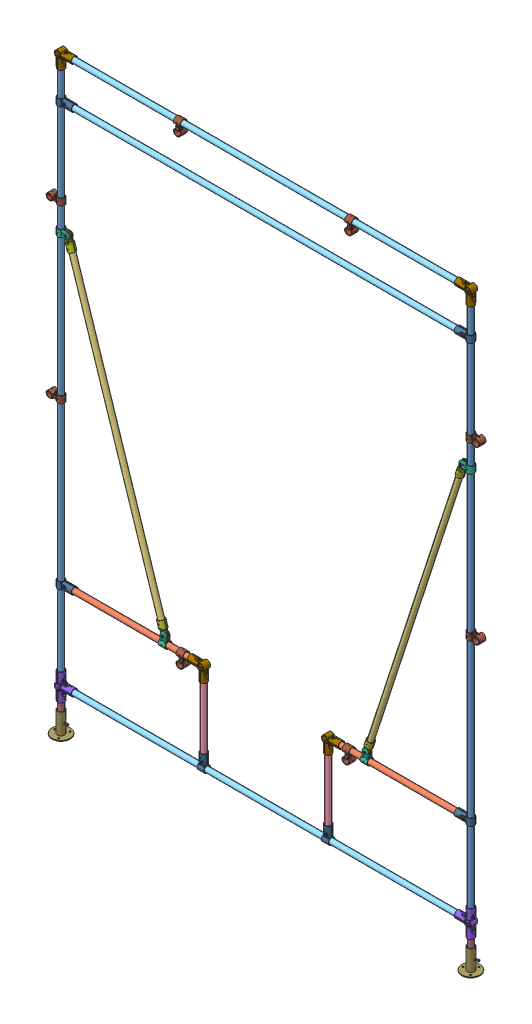
SolidWorks assembly Steel Tube Panel2, configuration Default. Lengths in mm.
Overall size (2121.41 2906.78 107.19).
47 component instances, 13 part files, 77 mates.
Components (placement in the parent):
- Height-1: Height [Default] at (0 2644.14 0) x (0 -1 0) z (0.644967 0 0.76421) size (2606.04 25.4 25.4)
- Horizonal Corner-1: Horizonal Corner [Default] at (1346.2 431.8 0) x (1 0 0) z (0 -0.094646 -0.995511) size (622.3 25.4 25.4)
- Lower Mounting Bar-1: Lower Mounting Bar [Default] at (1508.7506 501.6503 0) x (0.309017 0.951057 0) z (0.758734 -0.246528 0.602949) size (1460.5 25.4 25.4)
- Vertical Corner-1: Vertical Corner [Default] at (1308.1 38.1 0) x (0 1 0) z (-0.861516 0 -0.50773) size (355.6 25.4 25.4)
- Width-1: Width [Default] at (1968.5 0 0) x (-1 0 0) z (0 0.829168 0.559) size (1930.4 25.4 25.4)
- Adjustable_18deg-1: Adjustable_18deg [Default] at (1936.0393 1953.3743 -8.9201) x (-1 0 0) z (0 0 1) size (87.05 82.3 33.53)
  - Adjustable Connector Part 1-1: Adjustable Connector Part 1 [2534T33] at (-70.5607 28.1617 8.9201) size (68.33 33.53 33.53)
  - Adjustable Connector Part 2-1: Adjustable Connector Part 2 [2534T33] at (-46.1648 -5.4163 8.9201) x (0.309017 0.951057 0) z (0 0 1) size (75.66 33.46 33.53)
- Adjustable_72deg-1: Adjustable_72deg [Default] at (1469.3648 502.3607 8.9201) x (0 1 0) z (0 0 -1) size (115.94 55.2 33.53)
  - Adjustable Connector Part 1-1: Adjustable Connector Part 1 [2534T33] at (-70.5607 28.1617 8.9201) size (68.33 33.53 33.53)
  - Adjustable Connector Part 2-1: Adjustable Connector Part 2 [2534T33] at (-68.8327 17.2515 8.9201) x (0.951057 0.309017 0) z (0 0 1) size (75.66 33.46 33.53)
- 5way connector-1: 5way connector [2534T26] x (0 -1 0) z (0 0 -1) size (130.05 82.36 33.46)
- 5way connector-2: 5way connector [2534T26] at (2006.6 0 0) x (0 1 0) z (0 0 -1) size (130.05 82.36 33.46)
- Height-2: Height [Default] at (2006.6 2644.14 0) x (0 -1 0) z (0 0 1) size (2606.04 25.4 25.4)
- 3way connector-2: 3way connector [2534T24] at (2006.6 2682.24 0) x (-1 0 0) z (0 0 -1) size (81.85 81.28 33.46)
- 3way connector-3: 3way connector [2534T24] at (0 2682.24 0) size (81.85 81.28 33.46)
- Width-2: Width [Default] at (1968.5 2682.24 0) x (-1 0 0) z (0 0.006098 -0.999981) size (1930.4 25.4 25.4)
- Tee connector-1: Tee connector [2534T21] at (1308.1 0 0) x (1 0 0) z (0 0 -1) size (33.53 82.55 34.1)
- Tee connector-2: Tee connector [2534T21] at (2006.6 431.8 0) x (0 1 0) z (0 0 -1) size (33.53 82.55 34.1)
- 3way connector-4: 3way connector [2534T24] at (1308.1 431.8 0) size (81.85 81.28 33.46)
- Crossover-1: Crossover [2534T28] at (2006.6 1219.2 0) x (1 0 -0.000006) z (0 -1 0) size (74.17 39.33 39.33)
- Crossover-2: Crossover [2534T28] at (2006.6 2057.4 0) x (1 0 -0.000006) z (0 -1 0) size (74.17 39.33 39.33)
- Crossover-3: Crossover [2534T28] at (1422.4 2682.24 0) x (0 -1 -0.000006) z (-1 0 0) size (74.17 39.33 39.33)
- Tee connector-9: Tee connector [2534T21] at (0 2479.04 0) x (0 1 0) z (0 0 1) size (33.53 82.55 34.1)
- Tee connector-10: Tee connector [2534T21] at (2006.6 2479.04 0) x (0 -1 0) z (0 0 1) size (33.53 82.55 34.1)
- Width-3: Width [Default] at (38.1 2479.04 0) x (1 0 0) z (0 -0.966208 0.257766) size (1930.4 25.4 25.4)
- Crossover-13: Crossover [2534T28] at (584.2 2682.24 0) x (0 -1 -0.000006) z (1 0 0) size (74.17 39.33 39.33)
- Adjustable_18deg-5: Adjustable_18deg [Default] at (70.5607 1953.3743 8.9201) x (1 0 0) z (0 0 -1) size (87.05 82.3 33.53)
  - Adjustable Connector Part 1-1: Adjustable Connector Part 1 [2534T33] at (-70.5607 28.1617 8.9201) size (68.33 33.53 33.53)
  - Adjustable Connector Part 2-1: Adjustable Connector Part 2 [2534T33] at (-46.1648 -5.4163 8.9201) x (0.309017 0.951057 0) z (0 0 1) size (75.66 33.46 33.53)
- Lower Mounting Bar-5: Lower Mounting Bar [Default] at (497.8494 501.6503 0) x (-0.309017 0.951057 0) z (0.758734 0.246528 -0.602949) size (1460.5 25.4 25.4)
- Horizonal Corner-5: Horizonal Corner [Default] at (660.4 431.8 0) x (-1 0 0) z (0 0.094646 0.995511) size (622.3 25.4 25.4)
- Adjustable_72deg-5: Adjustable_72deg [Default] at (537.2352 502.3607 -8.9201) x (0 1 0) z (0 0 1) size (115.94 55.2 33.53)
  - Adjustable Connector Part 1-1: Adjustable Connector Part 1 [2534T33] at (-70.5607 28.1617 8.9201) size (68.33 33.53 33.53)
  - Adjustable Connector Part 2-1: Adjustable Connector Part 2 [2534T33] at (-68.8327 17.2515 8.9201) x (0.951057 0.309017 0) z (0 0 1) size (75.66 33.46 33.53)
- Tee connector-13: Tee connector [2534T21] at (0 431.8 0) x (0 -1 0) z (0 0 -1) size (33.53 82.55 34.1)
- 3way connector-8: 3way connector [2534T24] at (698.5 431.8 0) x (-1 0 0) z (0 0 -1) size (81.85 81.28 33.46)
- Vertical Corner-5: Vertical Corner [Default] at (698.5 38.1 0) x (0 1 0) z (-0.861516 0 0.50773) size (355.6 25.4 25.4)
- Tee connector-14: Tee connector [2534T21] at (698.5 0 -0.5732) x (-1 0 0) z (0 0 1) size (33.53 82.55 34.1)
- Crossover-18: Crossover [2534T28] at (0 2057.4 0) x (-1 0 -0.000006) z (0 1 0) size (74.17 39.33 39.33)
- Crossover-19: Crossover [2534T28] at (0 1219.2 0) x (-1 0 -0.000006) z (0 1 0) size (74.17 39.33 39.33)
- lil' feetie-1: lil' feetie [2534T82] at (2006.6 -207.772 0) x (0.972408 0 -0.233285) z (0 1 0) size (88.9 88.9 104.65)
- lil' legs-1: lil' legs [Default] at (2006.6 -190.5 0) x (0 1 0) z (0 0 1) size (152.4 25.4 25.4)
- lil' feetie-3: lil' feetie [2534T82] at (0 -207.772 0) x (1 0 0) z (0 1 0) size (88.9 88.9 104.65)
- lil' legs-3: lil' legs [Default] at (0 -190.5 0) x (0 1 0) z (-0.056771 0 0.998387) size (152.4 25.4 25.4)
- Crossover-20: Crossover [2534T28] at (1409.7 431.8 0) x (0 -1 -0.000006) z (-1 0 0) size (74.17 39.33 39.33)
- Crossover-21: Crossover [2534T28] at (596.9 431.8 0) x (0 -1 -0.000006) z (-1 0 0) size (74.17 39.33 39.33)
Mates (geometry in assembly coordinates):
- Concentric1: concentric anti-aligned: cylinder of Height-1 through (0 38.1 0) axis (0 1 0) radius 12.7; cylinder of 5way connector-1 through (0 65.024 0) axis (0 -1 0) radius 13.97
- Distance1: distance = 38.1 mm: point of 5way connector-1; plane of Height-1 through (0 38.1 0) normal (0 -1 0)
- Concentric2: concentric anti-aligned: cylinder of Width-1 through (38.1 0 0) axis (1 0 0) radius 12.7; cylinder of 5way connector-1 through (65.024 0 0) axis (-1 0 0) radius 13.97
- Distance2: distance = 38.1 mm: point of 5way connector-1; plane of Width-1 through (38.1 0 0) normal (-1 0 0)
- Distance3: distance = 38.1 mm anti-aligned: plane of Height-1 through (0 38.1 0) normal (0 -1 0); plane of assembly through (0 0 0) normal (0 1 0)
- Parallel2: parallel aligned: plane of Width-1 through (1968.5 0 0) normal (1 0 0); plane of assembly through (0 0 0) normal (1 0 0)
- Coincident9: coincident: point of 5way connector-1; plane of assembly
- Concentric3: concentric aligned: cylinder of Width-1 through (38.1 0 0) axis (1 0 0) radius 12.7; cylinder of 5way connector-2 through (1941.576 0 0) axis (1 0 0) radius 13.97
- Distance4: distance = 38.1 mm: point of 5way connector-2; plane of Width-1 through (1968.5 0 0) normal (1 0 0)
- Parallel3: parallel anti-aligned: plane of 5way connector-2 through (2006.6 -65.024 0) normal (0 -1 0); plane of assembly through (0 0 0) normal (0 1 0)
- Concentric4: concentric anti-aligned: cylinder of 5way connector-2 through (2006.6 65.024 0) axis (0 -1 0) radius 13.97; cylinder of Height-2 through (2006.6 38.1 0) axis (0 1 0) radius 12.7
- Distance5: distance = 38.1 mm: point of 5way connector-2; plane of Height-2 through (2006.6 38.1 0) normal (0 -1 0)
- Concentric6: concentric aligned: cylinder of Height-2 through (2006.6 38.1 0) axis (0 1 0) radius 12.7; cylinder of 3way connector-2 through (2006.6 2617.724 0) axis (0 1 0) radius 13.97
- Coincident10: coincident: point of 5way connector-1; plane of assembly
- Distance6: distance = 38.1 mm: point of 3way connector-2; plane of Height-2 through (2006.6 2644.14 0) normal (0 1 0)
- Parallel5: parallel anti-aligned: plane of 3way connector-2 through (1942.084 2682.24 0) normal (-1 0 0); plane of assembly through (0 0 0) normal (1 0 0)
- Concentric7: concentric aligned: cylinder of Height-1 through (0 38.1 0) axis (0 1 0) radius 12.7; cylinder of 3way connector-3 through (0 2617.724 0) axis (0 1 0) radius 13.97
- Distance7: distance = 38.1 mm: point of 3way connector-3; plane of Height-1 through (0 2644.14 0) normal (0 1 0)
- Parallel6: parallel aligned: plane of 3way connector-3 through (64.516 2682.24 0) normal (1 0 0); plane of assembly through (0 0 0) normal (1 0 0)
- Concentric8: concentric anti-aligned: cylinder of 3way connector-3 through (64.516 2682.24 0) axis (-1 0 0) radius 13.97; cylinder of Width-2 through (38.1 2682.24 0) axis (1 0 0) radius 12.7
- Distance8: distance = 38.1 mm: point of 3way connector-3; plane of Width-2 through (38.1 2682.24 0) normal (-1 0 0)
- Concentric9: concentric aligned: cylinder of Width-1 through (38.1 0 0) axis (1 0 0) radius 12.7; cylinder of Tee connector-1 through (1291.336 0 0) axis (1 0 0) radius 13.97
- Parallel7: parallel aligned: plane of Tee connector-1 through (1308.1 65.786 0) normal (0 1 0); plane of assembly through (0 0 0) normal (0 1 0)
- Concentric10: concentric aligned: cylinder of Height-2 through (2006.6 38.1 0) axis (0 1 0) radius 12.7; cylinder of Tee connector-2 through (2006.6 415.036 0) axis (0 1 0) radius 13.97
- Parallel8: parallel anti-aligned: plane of Tee connector-2 through (1940.814 431.8 0) normal (-1 0 0); plane of assembly through (0 0 0) normal (1 0 0)
- Concentric11: concentric anti-aligned: cylinder of Horizonal Corner-1 through (1968.5 431.8 0) axis (-1 0 0) radius 12.7; cylinder of Tee connector-2 through (1940.814 431.8 0) axis (1 0 0) radius 13.97
- Distance9: distance = 38.1 mm: point of Tee connector-2; plane of Horizonal Corner-1 through (1968.5 431.8 0) normal (1 0 0)
- Concentric12: concentric aligned: cylinder of Horizonal Corner-1 through (1968.5 431.8 0) axis (-1 0 0) radius 12.7; cylinder of 3way connector-4 through (1372.616 431.8 0) axis (-1 0 0) radius 13.97
- Parallel9: parallel anti-aligned: plane of 3way connector-4 through (1308.1 367.284 0) normal (0 -1 0); plane of assembly through (0 0 0) normal (0 1 0)
- Concentric13: concentric anti-aligned: cylinder of Vertical Corner-1 through (1308.1 393.7 0) axis (0 -1 0) radius 12.7; cylinder of 3way connector-4 through (1308.1 367.284 0) axis (0 1 0) radius 13.97
- Distance10: distance = 38.1 mm: point of 3way connector-4; plane of Horizonal Corner-1 through (1346.2 431.8 0) normal (-1 0 0)
- Distance11: distance = 38.1 mm: point of 3way connector-4; plane of Vertical Corner-1 through (1308.1 393.7 0) normal (0 1 0)
- Concentric14: concentric aligned: cylinder of Vertical Corner-1 through (1308.1 393.7 0) axis (0 -1 0) radius 12.7; cylinder of Tee connector-1 through (1308.1 65.786 0) axis (0 -1 0) radius 13.97
- Distance12: distance = 38.1 mm: point of Tee connector-1; plane of Vertical Corner-1 through (1308.1 38.1 0) normal (0 -1 0)
- Concentric15: concentric aligned: cylinder of Horizonal Corner-1 through (1968.5 431.8 0) axis (-1 0 0) radius 12.7; cylinder of Adjustable_72deg-1/Adjustable Connector Part 1-1 through (1514.2914 431.8 0) axis (-1 0 0) radius 13.97
- Concentric16: concentric anti-aligned: cylinder of Adjustable_18deg-1/Adjustable Connector Part 1-1 through (2006.6 1941.9776 0) axis (0 -1 0) radius 13.97; cylinder of Height-2 through (2006.6 38.1 0) axis (0 1 0) radius 12.7
- Concentric17: concentric aligned: cylinder of Lower Mounting Bar-1 through (1960.0699 1890.6683 0) axis (-0.309017 -0.951057 0) radius 12.7; cylinder of Adjustable_18deg-1/Adjustable Connector Part 2-1 through (1964.4653 1904.1961 0) axis (-0.309017 -0.951057 0) radius 13.97
- Concentric18: concentric anti-aligned: cylinder of Lower Mounting Bar-1 through (1960.0699 1890.6683 0) axis (-0.309017 -0.951057 0) radius 12.7; cylinder of Adjustable_72deg-1/Adjustable Connector Part 2-1 through (1504.3551 488.1224 0) axis (0.309017 0.951057 0) radius 13.97
- Distance13: distance = 25.4 mm anti-aligned: plane of Adjustable_72deg-1/Adjustable Connector Part 2-1 through (1516.5996 525.8071 0) normal (0.309017 0.951057 0); plane of Lower Mounting Bar-1 through (1508.7506 501.6503 0) normal (-0.309017 -0.951057 0)
- Distance14: distance = 25.4 mm anti-aligned: plane of Adjustable_18deg-1/Adjustable Connector Part 2-1 through (1952.2209 1866.5115 0) normal (-0.309017 -0.951057 0); plane of Lower Mounting Bar-1 through (1960.0699 1890.6683 0) normal (0.309017 0.951057 0)
- Concentric20: concentric anti-aligned: cylinder of Height-2 through (2006.6 38.1 0) axis (0 1 0) radius 12.7; cylinder of Crossover-1 through (2006.6 1235.202 0) axis (0 -1 0) radius 13.97
- Distance15: distance = 1219.2 mm: point of Crossover-1; point of 5way connector-2
- Concentric21: concentric aligned: cylinder of Height-2 through (2006.6 38.1 0) axis (0 1 0) radius 12.7; cylinder of Crossover-2 through (2006.6 2041.398 0) axis (0 1 0) radius 13.97
- Distance16: distance = 2057.4 mm: point of Crossover-2; point of 5way connector-2
- Concentric22: concentric aligned: cylinder of Width-2 through (38.1 2682.24 0) axis (1 0 0) radius 12.7; cylinder of Crossover-3 through (1406.398 2682.24 0) axis (1 0 0) radius 13.97
- Distance17: distance = 584.2 mm: point of Crossover-3; point of 3way connector-2
- Concentric23: concentric aligned: cylinder of Height-2 through (2006.6 38.1 0) axis (0 1 0) radius 12.7; cylinder of Tee connector-10 through (2006.6 2462.276 0) axis (0 1 0) radius 13.97
- Parallel13: parallel anti-aligned: plane of Tee connector-10 through (1940.814 2479.04 0) normal (-1 0 0); plane of assembly through (0 0 0) normal (1 0 0)
- Concentric24: concentric anti-aligned: cylinder of Tee connector-10 through (1940.814 2479.04 0) axis (1 0 0) radius 13.97; cylinder of Width-3 through (1968.5 2479.04 0) axis (-1 0 0) radius 12.7
- Distance18: distance = 38.1 mm: point of Tee connector-10; plane of Width-3 through (1968.5 2479.04 0) normal (1 0 0)
- Concentric25: concentric anti-aligned: cylinder of Height-1 through (0 38.1 0) axis (0 1 0) radius 12.7; cylinder of Tee connector-9 through (0 2495.804 0) axis (0 -1 0) radius 13.97
- Parallel15: parallel aligned: plane of Tee connector-9 through (65.786 2479.04 0) normal (1 0 0); plane of assembly through (0 0 0) normal (1 0 0)
- Concentric26: concentric aligned: cylinder of Tee connector-9 through (65.786 2479.04 0) axis (-1 0 0) radius 13.97; cylinder of Width-3 through (1968.5 2479.04 0) axis (-1 0 0) radius 12.7
- Distance19: distance = 203.2 mm: point of Tee connector-9; point of 3way connector-3
- Distance21: distance = 1.778 mm: line of Crossover-2 through (2047.2374 2040.636 1.778) axis (0 1 0); plane of assembly
- Distance20: distance = 1.778 mm: line of Crossover-1 through (2047.2374 1202.436 1.778) axis (0 1 0); plane of assembly
- Distance22: distance = 1.778 mm: line of Crossover-3 through (1405.636 2641.6026 1.778) axis (1 0 0); plane of assembly
- Concentric27: concentric anti-aligned: cylinder of Height-1 through (0 38.1 0) axis (0 1 0) radius 12.7; cylinder of Crossover-19 through (0 1235.202 0) axis (0 -1 0) radius 13.97
- Concentric28: concentric anti-aligned: cylinder of Height-1 through (0 38.1 0) axis (0 1 0) radius 12.7; cylinder of Crossover-18 through (0 2073.402 0) axis (0 -1 0) radius 13.97
- Distance23: distance = 1.778 mm: plane of assembly through (0 0 0) normal (0 0 1); line of Crossover-18 through (-40.6374 2074.164 1.778) axis (0 -1 0)
- Distance24: distance = 1.778 mm: plane of assembly through (0 0 0) normal (0 0 1); line of Crossover-19 through (-40.6374 1235.964 1.778) axis (0 -1 0)
- Distance25: distance = 1219.2 mm: point of Crossover-19; point of assembly
- Distance26: distance = 2057.4 mm: point of Crossover-18; point of assembly
- Concentric29: concentric anti-aligned: cylinder of 5way connector-2 through (2006.6 -65.024 0) axis (0 1 0) radius 13.97; cylinder of lil' legs-1 through (2006.6 -38.1 0) axis (0 -1 0) radius 12.7
- Concentric30: concentric aligned: cylinder of lil' feetie-1 through (2006.6 -103.124 0) axis (0 -1 0) radius 15.367; cylinder of lil' legs-1 through (2006.6 -38.1 0) axis (0 -1 0) radius 12.7
- Distance27: distance = 38.1 mm: point of 5way connector-2; plane of lil' legs-1 through (2006.6 -38.1 0) normal (0 1 0)
- Distance28: distance = 38.1 mm anti-aligned: plane of lil' feetie-1 through (2006.6 -103.124 0) normal (0 1 0); plane of 5way connector-2 through (2006.6 -65.024 0) normal (0 -1 0)
- Concentric31: concentric anti-aligned: cylinder of 5way connector-1 through (0 -65.024 0) axis (0 1 0) radius 13.97; cylinder of lil' legs-3 through (0 -38.1 0) axis (0 -1 0) radius 12.7
- Concentric32: concentric aligned: cylinder of lil' feetie-3 through (0 -103.124 0) axis (0 -1 0) radius 15.367; cylinder of lil' legs-3 through (0 -38.1 0) axis (0 -1 0) radius 12.7
- Distance30: distance = 38.1 mm: point of assembly; plane of lil' legs-3 through (0 -38.1 0) normal (0 1 0)
- Distance31: distance = 38.1 mm anti-aligned: plane of 5way connector-1 through (0 -65.024 0) normal (0 -1 0); plane of lil' feetie-3 through (0 -103.124 0) normal (0 1 0)
- Concentric33: concentric anti-aligned: cylinder of Horizonal Corner-5 through (38.1 431.8 0) axis (1 0 0) radius 12.7; cylinder of Crossover-21 through (612.902 431.8 0) axis (-1 0 0) radius 13.97
- Distance32: distance = 101.6 mm: point of Crossover-21; point of 3way connector-8
- Concentric35: concentric anti-aligned: cylinder of Horizonal Corner-1 through (1968.5 431.8 0) axis (-1 0 0) radius 12.7; cylinder of Crossover-20 through (1393.698 431.8 0) axis (1 0 0) radius 13.97
- Distance33: distance = 101.6 mm: point of Crossover-20; point of 3way connector-4
- Distance34: distance = 1.778 mm: line of Crossover-20 through (1392.936 391.1626 1.778) axis (1 0 0); plane of assembly
- Distance35: distance = 1.778 mm: line of Crossover-21 through (580.136 391.1626 1.778) axis (1 0 0); plane of assembly
